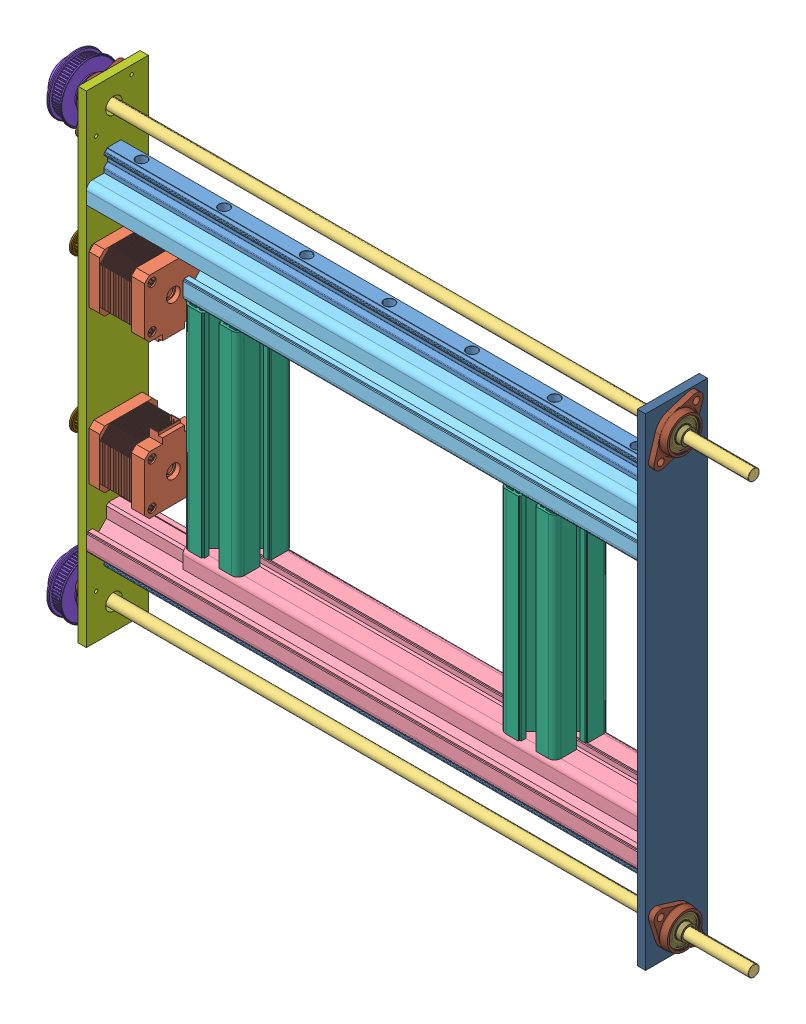
SolidWorks assembly Mesa, configuration Predeterminado. Lengths in mm.
Overall size (500 363.97 51.97).
38 component instances, 15 part files, 62 mates.
Components (placement in the parent):
- Mesa-1: Mesa [Predeterminado] at origin size (412 330 4) (hidden)
- Copia de HGR15R Rail^Mesa-1: Copia de HGR15R Rail^Mesa [HGR15R400CE20] at (0 282 -20) x (0 0 1) z (-1 0 0) size (15 15 400) (virtual)
- Copia de HGR15R Rail^Mesa-2: Copia de HGR15R Rail^Mesa [HGR15R400CE20] at (0 48 -20) x (0 0 -1) z (-1 0 0) size (15 15 400) (virtual)
- Nema_17HS4401-S^Mesa-1: Nema_17HS4401-S^Mesa [Varsayılan] at (40.2 220.5 -23) x (0 0 -1) z (-1 0 0) size (42 48 63.23) (virtual)
- LeadScrew 8mm x 2mmPitch^Mesa-1: LeadScrew 8mm x 2mmPitch^Mesa [Default] at (464.65 9 -20) x (0 1 0) z (1 0 0) size (8 8 500) (virtual)
- LeadScrew 8mm x 2mmPitch^Mesa-2: LeadScrew 8mm x 2mmPitch^Mesa [Default] at (464.65 321 -20) x (0 -1 0) z (1 0 0) size (8 8 500) (virtual)
- yn_4040^Mesa-1: yn_4040^Mesa [Default] at (400 68 -20) x (0 1 0) z (-1 0 0) size (40 40 400) (virtual)
- yp_4040^Mesa-3: yp_4040^Mesa [Default] at (400 262 -20) x (0 1 0) z (-1 0 0) size (40 40 400) (virtual)
- xp_4040^Mesa-2: xp_4040^Mesa [Default] at (90 242 -20) x (-1 0 0) z (0 -1 0) size (40 40 154) (virtual)
- soporte_motores^Mesa-1: soporte_motores^Mesa [Predeterminado] at (-6 340 0) x (0 1 0) z (1 0 0) size (350 45 6) (virtual)
- farola^Mesa-1: farola^Mesa [Predeterminado] at (450.1962 5.1009 28.2108) x (0.008727 0.999962 0) z (0 0 1) size (325 500 6) (hidden, virtual)
- GT2_60T_8_6^Mesa-2: GT2_60T_8_6^Mesa [Default] at (-27.85 321 -20) x (0 0 1) z (1 0 0) size (42 42 18) (virtual)
- GT2_20T^Mesa-1: GT2_20T^Mesa [Конфигурация1] at (-11.4 220.5 -23) x (-1 0 0) z (0 0 1) size (16 16 16) (virtual)
- GT2_60T_8_6^Mesa-3: GT2_60T_8_6^Mesa [Default] at (-27.85 9 -20) x (0 0 -1) z (1 0 0) size (42 42 18) (virtual)
- Nema_17HS4401-S^Mesa-2: Nema_17HS4401-S^Mesa [Varsayılan] at (40.2 109.5 -23) x (0 0 1) z (-1 0 0) size (42 48 63.23) (virtual)
- GT2_20T^Mesa-2: GT2_20T^Mesa [Конфигурация1] at (-11.4 109.5 -23) x (-1 0 0) z (0 1 0) size (16 16 16) (virtual)
- soporte_frontal^Mesa-1: soporte_frontal^Mesa [Predeterminado] at (400 340 0) x (0 1 0) z (1 0 0) size (350 45 6) (virtual)
- KFL08^Mesa-3: KFL08^Mesa [Varsayılan] at (-6 9 -20) x (0 0.707107 0.707107) z (0 -0.707107 0.707107) size (46.5 11.35 27) (virtual)
  - FLANGE-1: FLANGE [Default] at origin size (46.5 8.5 27)
  - BEARING-1: BEARING [Default] at (0 4 0) x (1 0 0) z (0 -1 0) size (22 22 10.85)
  - socket set screw cone point_am-1: socket set screw cone point_am [B18.3.6M - M2.5 x 0.45 x 2 Hex Socket Cone Pt. SS --S] at (0 9.425 5.45) x (0 0 -1) z (1 0 0) size (2 2.5 2.5)
  - socket set screw cone point_am-2: socket set screw cone point_am [B18.3.6M - M2.5 x 0.45 x 2 Hex Socket Cone Pt. SS --S] at (5.45 9.425 0) x (-1 0 0) z (0 0 -1) size (2 2.5 2.5)
- KFL08^Mesa-2: KFL08^Mesa [Varsayılan] at (-6 321 -20) x (0 -0.707107 0.707107) z (0 -0.707107 -0.707107) size (46.5 11.35 27) (virtual)
  - FLANGE-1: FLANGE [Default] at origin size (46.5 8.5 27)
  - BEARING-1: BEARING [Default] at (0 4 0) x (1 0 0) z (0 -1 0) size (22 22 10.85)
  - socket set screw cone point_am-1: socket set screw cone point_am [B18.3.6M - M2.5 x 0.45 x 2 Hex Socket Cone Pt. SS --S] at (0 9.425 5.45) x (0 0 -1) z (1 0 0) size (2 2.5 2.5)
  - socket set screw cone point_am-2: socket set screw cone point_am [B18.3.6M - M2.5 x 0.45 x 2 Hex Socket Cone Pt. SS --S] at (5.45 9.425 0) x (-1 0 0) z (0 0 -1) size (2 2.5 2.5)
- KFL08^Mesa-4: KFL08^Mesa [Varsayılan] at (406 9 -20) x (0 -0.707107 -0.707107) z (0 -0.707107 0.707107) size (46.5 11.35 27) (virtual)
  - FLANGE-1: FLANGE [Default] at origin size (46.5 8.5 27)
  - BEARING-1: BEARING [Default] at (0 4 0) x (1 0 0) z (0 -1 0) size (22 22 10.85)
  - socket set screw cone point_am-1: socket set screw cone point_am [B18.3.6M - M2.5 x 0.45 x 2 Hex Socket Cone Pt. SS --S] at (0 9.425 5.45) x (0 0 -1) z (1 0 0) size (2 2.5 2.5)
  - socket set screw cone point_am-2: socket set screw cone point_am [B18.3.6M - M2.5 x 0.45 x 2 Hex Socket Cone Pt. SS --S] at (5.45 9.425 0) x (-1 0 0) z (0 0 -1) size (2 2.5 2.5)
- KFL08^Mesa-5: KFL08^Mesa [Varsayılan] at (406 321 -20) x (0 0.707107 -0.707107) z (0 -0.707107 -0.707107) size (46.5 11.35 27) (virtual)
  - FLANGE-1: FLANGE [Default] at origin size (46.5 8.5 27)
  - BEARING-1: BEARING [Default] at (0 4 0) x (1 0 0) z (0 -1 0) size (22 22 10.85)
  - socket set screw cone point_am-1: socket set screw cone point_am [B18.3.6M - M2.5 x 0.45 x 2 Hex Socket Cone Pt. SS --S] at (0 9.425 5.45) x (0 0 -1) z (1 0 0) size (2 2.5 2.5)
  - socket set screw cone point_am-2: socket set screw cone point_am [B18.3.6M - M2.5 x 0.45 x 2 Hex Socket Cone Pt. SS --S] at (5.45 9.425 0) x (-1 0 0) z (0 0 -1) size (2 2.5 2.5)
- xp_4040^Mesa-3: xp_4040^Mesa [Default] at (320 242 -20) x (-1 0 0) z (0 -1 0) size (40 40 154) (virtual)
Mates (geometry in assembly coordinates):
- Coincidente34: coincident anti-aligned: plane of Mesa-1 through (0 0 0) normal (0 0 -1); plane of yn_4040^Mesa-1 through (0 52.5 0) normal (0 0 1)
- Coincidente35: coincident aligned: plane of Mesa-1 through (0 0 4) normal (-1 0 0); plane of yn_4040^Mesa-1 through (0 83.5 -35.5) normal (-1 0 0)
- Coincidente36: coincident anti-aligned: plane of Mesa-1 through (0 0 0) normal (0 0 -1); plane of yp_4040^Mesa-3 through (0 246.5 0) normal (0 0 1)
- Coincidente37: coincident aligned: plane of Mesa-1 through (0 0 4) normal (-1 0 0); plane of yp_4040^Mesa-3 through (0 277.5 -35.5) normal (-1 0 0)
- Coincidente38: coincident anti-aligned: plane of Copia de HGR15R Rail^Mesa-2 through (400 48 -13) normal (0 1 0); plane of yn_4040^Mesa-1 through (0 48 -23.9656) normal (0 -1 0)
- Coincidente39: coincident aligned: plane of Copia de HGR15R Rail^Mesa-2 through (0 44.9142 -26.5) normal (-1 0 0); plane of yn_4040^Mesa-1 through (0 83.5 -35.5) normal (-1 0 0)
- Coincidente40: coincident anti-aligned: plane of Copia de HGR15R Rail^Mesa-1 through (400 282 -27) normal (0 -1 0); plane of yp_4040^Mesa-3 through (0 282 -23.9656) normal (0 1 0)
- Coincidente41: coincident aligned: plane of Copia de HGR15R Rail^Mesa-1 through (0 285.0858 -13.5) normal (-1 0 0); plane of yp_4040^Mesa-3 through (0 277.5 -35.5) normal (-1 0 0)
- Distancia9: distance = 12.5 mm aligned: plane of Copia de HGR15R Rail^Mesa-1 through (400 282.5 -27.5) normal (0 0 -1); plane of yp_4040^Mesa-3 through (0 277.5 -40) normal (0 0 -1)
- Distancia10: distance = 12.5 mm aligned: plane of Copia de HGR15R Rail^Mesa-2 through (400 47.5 -27.5) normal (0 0 -1); plane of yn_4040^Mesa-1 through (0 52.5 -40) normal (0 0 -1)
- Distancia13: distance = 48 mm aligned: plane of yn_4040^Mesa-1 through (0 48 -16.0344) normal (0 -1 0); plane of Mesa-1 through (0 0 4) normal (0 -1 0)
- Distancia15: distance = 154 mm anti-aligned: plane of yn_4040^Mesa-1 through (0 88 -16.0344) normal (0 1 0); plane of yp_4040^Mesa-3 through (0 242 -16.0344) normal (0 -1 0)
- Coincidente49: coincident anti-aligned: plane of yp_4040^Mesa-3 through (0 277.5 -35.5) normal (-1 0 0); plane of soporte_motores^Mesa-1 through (0 340 0) normal (1 0 0)
- Coincidente50: coincident aligned: plane of yp_4040^Mesa-3 through (0 277.5 0) normal (0 0 1); plane of soporte_motores^Mesa-1 through (0 -10 0) normal (0 0 1)
- Distancia18: distance = 58 mm aligned: plane of yp_4040^Mesa-3 through (0 282 -16.0344) normal (0 1 0); plane of soporte_motores^Mesa-1 through (0 340 -45) normal (0 1 0)
- Coincidente52: coincident anti-aligned: plane of soporte_motores^Mesa-1 through (-6 340 0) normal (-1 0 0); plane of KFL08^Mesa-2/FLANGE-1 through (-6 308.0953 -7.0953) normal (1 0 0)
- Concéntrica1: concentric aligned: cylinder of soporte_motores^Mesa-1 through (-6 321 -20) axis (1 0 0) radius 6; cylinder of KFL08^Mesa-2/BEARING-1 through (-6.5 321 -20) axis (1 0 0) radius 4
- Concéntrica2: concentric anti-aligned: cylinder of soporte_motores^Mesa-1 through (-6 333.9047 -32.9047) axis (1 0 0) radius 1.25; cylinder of KFL08^Mesa-2/FLANGE-1 through (-10 333.9047 -32.9047) axis (-1 0 0) radius 2.5
- Coincidente53: coincident anti-aligned: plane of soporte_motores^Mesa-1 through (-6 340 0) normal (-1 0 0); plane of KFL08^Mesa-3/FLANGE-1 through (-6 21.9047 -7.0953) normal (1 0 0)
- Concéntrica3: concentric aligned: cylinder of soporte_motores^Mesa-1 through (-6 9 -20) axis (1 0 0) radius 6; cylinder of KFL08^Mesa-3/BEARING-1 through (-6.5 9 -20) axis (1 0 0) radius 4
- Concéntrica4: concentric anti-aligned: cylinder of soporte_motores^Mesa-1 through (-6 21.9047 -7.0953) axis (1 0 0) radius 1.25; cylinder of KFL08^Mesa-3/FLANGE-1 through (-10 21.9047 -7.0953) axis (-1 0 0) radius 2.5
- Concéntrica5: concentric aligned: cylinder of LeadScrew 8mm x 2mmPitch^Mesa-1 through (-35.35 9 -20) axis (1 0 0) radius 4; cylinder of KFL08^Mesa-3/BEARING-1 through (-6.5 9 -20) axis (1 0 0) radius 4
- Concéntrica6: concentric aligned: cylinder of LeadScrew 8mm x 2mmPitch^Mesa-2 through (-35.35 321 -20) axis (1 0 0) radius 4; cylinder of KFL08^Mesa-2/BEARING-1 through (-6.5 321 -20) axis (1 0 0) radius 4
- Concéntrica7: concentric aligned: circle of LeadScrew 8mm x 2mmPitch^Mesa-2; circle of GT2_60T_8_6^Mesa-2
- Coincidente54: coincident anti-aligned: plane of KFL08^Mesa-2/BEARING-1 through (-17.35 317.9594 -23.0406) normal (-1 0 0); plane of GT2_60T_8_6^Mesa-2 through (-17.35 321 -20) normal (1 0 0)
- Coincidente55: coincident aligned: plane of LeadScrew 8mm x 2mmPitch^Mesa-2 through (-35.35 321 -20) normal (-1 0 0); plane of GT2_60T_8_6^Mesa-2 through (-35.35 321 -20) normal (-1 0 0)
- Coincidente56: coincident anti-aligned: plane of Nema_17HS4401-S^Mesa-1 through (0 220.5 -23) normal (-1 0 0); plane of soporte_motores^Mesa-1 through (0 340 0) normal (1 0 0)
- Distancia19: distance = 2 mm aligned: plane of Nema_17HS4401-S^Mesa-1 through (30.7 238 -2) normal (0 0 1); plane of soporte_motores^Mesa-1 through (0 -10 0) normal (0 0 1)
- Distancia20: distance = 15 mm anti-aligned: plane of Nema_17HS4401-S^Mesa-1 through (30.7 241.5 -5.5) normal (0 1 0); plane of yp_4040^Mesa-3 through (0 256.5 -20) normal (0 -1 0)
- Concéntrica8: concentric anti-aligned: cylinder of Nema_17HS4401-S^Mesa-1 through (-23 220.5 -23) axis (1 0 0) radius 2.5; cylinder of GT2_20T^Mesa-1 through (-11.4 220.5 -23) axis (-1 0 0) radius 2.5
- Coincidente59: coincident aligned: plane of GT2_60T_8_6^Mesa-2 through (-18.85 321 -20) normal (-1 0 0); plane of GT2_20T^Mesa-1 through (-18.85 220.5 -23) normal (-1 0 0)
- Concéntrica9: concentric anti-aligned: cylinder of LeadScrew 8mm x 2mmPitch^Mesa-1 through (-35.35 9 -20) axis (1 0 0) radius 4; cylinder of GT2_60T_8_6^Mesa-3 through (2.15 9 -20) axis (-1 0 0) radius 4
- Coincidente60: coincident anti-aligned: plane of KFL08^Mesa-3/BEARING-1 through (-17.35 5.9594 -16.9594) normal (-1 0 0); plane of GT2_60T_8_6^Mesa-3 through (-17.35 9 -20) normal (1 0 0)
- Coincidente61: coincident aligned: plane of LeadScrew 8mm x 2mmPitch^Mesa-1 through (-35.35 9 -20) normal (-1 0 0); plane of GT2_60T_8_6^Mesa-3 through (-35.35 9 -20) normal (-1 0 0)
- Coincidente62: coincident anti-aligned: plane of soporte_motores^Mesa-1 through (0 340 0) normal (1 0 0); plane of Nema_17HS4401-S^Mesa-2 through (0 109.5 -23) normal (-1 0 0)
- Distancia21: distance = 15 mm anti-aligned: plane of Nema_17HS4401-S^Mesa-2 through (30.7 88.5 -40.5) normal (0 -1 0); plane of yn_4040^Mesa-1 through (0 73.5 -20) normal (0 1 0)
- Distancia22: distance = 2 mm aligned: plane of Nema_17HS4401-S^Mesa-2 through (30.7 92 -2) normal (0 0 1); plane of soporte_motores^Mesa-1 through (0 -10 0) normal (0 0 1)
- Concéntrica10: concentric anti-aligned: cylinder of Nema_17HS4401-S^Mesa-2 through (-23 109.5 -23) axis (1 0 0) radius 2.5; cylinder of GT2_20T^Mesa-2 through (-11.4 109.5 -23) axis (-1 0 0) radius 2.5
- Coincidente65: coincident aligned: plane of GT2_60T_8_6^Mesa-3 through (-18.85 9 -20) normal (-1 0 0); plane of GT2_20T^Mesa-2 through (-18.85 109.5 -23) normal (-1 0 0)
- Coincidente66: coincident anti-aligned: plane of yn_4040^Mesa-1 through (400 83.5 -35.5) normal (1 0 0); plane of soporte_frontal^Mesa-1 through (400 340 0) normal (-1 0 0)
- Coincidente67: coincident aligned: plane of yn_4040^Mesa-1 through (0 52.5 0) normal (0 0 1); plane of soporte_frontal^Mesa-1 through (406 -10 0) normal (0 0 1)
- Concéntrica11: concentric aligned: cylinder of LeadScrew 8mm x 2mmPitch^Mesa-1 through (-35.35 9 -20) axis (1 0 0) radius 4; cylinder of soporte_frontal^Mesa-1 through (400 9 -20) axis (1 0 0) radius 6
- Coincidente68: coincident anti-aligned: plane of soporte_frontal^Mesa-1 through (406 340 0) normal (1 0 0); plane of KFL08^Mesa-5/FLANGE-1 through (406 333.9047 -32.9047) normal (-1 0 0)
- Coincidente69: coincident anti-aligned: plane of soporte_frontal^Mesa-1 through (406 340 0) normal (1 0 0); plane of KFL08^Mesa-4/FLANGE-1 through (406 -3.9047 -32.9047) normal (-1 0 0)
- Concéntrica12: concentric aligned: cylinder of soporte_frontal^Mesa-1 through (400 21.9047 -7.0953) axis (1 0 0) radius 1.25; cylinder of KFL08^Mesa-4/FLANGE-1 through (410 21.9047 -7.0953) axis (1 0 0) radius 2.5
- Concéntrica13: concentric anti-aligned: cylinder of LeadScrew 8mm x 2mmPitch^Mesa-1 through (-35.35 9 -20) axis (1 0 0) radius 4; cylinder of KFL08^Mesa-4/BEARING-1 through (406.5 9 -20) axis (-1 0 0) radius 4
- Concéntrica14: concentric anti-aligned: cylinder of LeadScrew 8mm x 2mmPitch^Mesa-2 through (-35.35 321 -20) axis (1 0 0) radius 4; cylinder of KFL08^Mesa-5/BEARING-1 through (406.5 321 -20) axis (-1 0 0) radius 4
- Concéntrica15: concentric aligned: cylinder of soporte_frontal^Mesa-1 through (400 308.0953 -7.0953) axis (1 0 0) radius 1.25; cylinder of KFL08^Mesa-5/FLANGE-1 through (410 308.0953 -7.0953) axis (1 0 0) radius 2.5
- Paralelo1: parallel aligned: plane of LeadScrew 8mm x 2mmPitch^Mesa-1 through (-25.35 6 -13.5951) normal (0 -1 0); plane of GT2_60T_8_6^Mesa-3 through (-31.6 -4 -20) normal (0 -1 0)
- Paralelo2: parallel aligned: plane of soporte_motores^Mesa-1 through (0 -10 -45) normal (0 -1 0); plane of GT2_60T_8_6^Mesa-3 through (-31.6 -4 -20) normal (0 -1 0)
- Paralelo3: parallel aligned: plane of LeadScrew 8mm x 2mmPitch^Mesa-2 through (-25.35 324 -26.4049) normal (0 1 0); plane of GT2_60T_8_6^Mesa-2 through (-31.6 334 -20) normal (0 1 0)
- Paralelo4: parallel aligned: plane of soporte_motores^Mesa-1 through (0 340 -45) normal (0 1 0); plane of GT2_60T_8_6^Mesa-2 through (-31.6 334 -20) normal (0 1 0)
- Paralelo5: parallel aligned: plane of Nema_17HS4401-S^Mesa-1 through (-6 218.6296 -21.3412) normal (0 -1 0); plane of GT2_20T^Mesa-1 through (-15.4 213 -23) normal (0 -1 0)
- Paralelo6: parallel aligned: plane of soporte_motores^Mesa-1 through (0 -10 0) normal (0 0 1); plane of GT2_20T^Mesa-1 through (-15.4 220.5 -15.5) normal (0 0 1)
- Paralelo7: parallel aligned: plane of Nema_17HS4401-S^Mesa-2 through (-6 111.3704 -24.6588) normal (0 1 0); plane of GT2_20T^Mesa-2 through (-15.4 117 -23) normal (0 1 0)
- Paralelo8: parallel aligned: plane of soporte_motores^Mesa-1 through (0 -10 0) normal (0 0 1); plane of GT2_20T^Mesa-2 through (-15.4 109.5 -15.5) normal (0 0 1)
- Coincidente76: coincident anti-aligned: plane of yp_4040^Mesa-3 through (0 242 -16.0344) normal (0 -1 0); plane of xp_4040^Mesa-2 through (74.5 242 -35.5) normal (0 1 0)
- Coincidente77: coincident aligned: plane of yp_4040^Mesa-3 through (0 246.5 0) normal (0 0 1); plane of xp_4040^Mesa-2 through (105.5 88 0) normal (0 0 1)
- Distancia23: distance = 70 mm anti-aligned: plane of soporte_motores^Mesa-1 through (0 340 0) normal (1 0 0); plane of xp_4040^Mesa-2 through (70 88 -16.0344) normal (-1 0 0)
- Coincidente79: coincident aligned: plane of yp_4040^Mesa-3 through (0 246.5 0) normal (0 0 1); plane of xp_4040^Mesa-3 through (335.5 88 0) normal (0 0 1)
- Coincidente80: coincident anti-aligned: plane of yp_4040^Mesa-3 through (0 242 -16.0344) normal (0 -1 0); plane of xp_4040^Mesa-3 through (304.5 242 -35.5) normal (0 1 0)
- Distancia24: distance = 60 mm anti-aligned: plane of xp_4040^Mesa-3 through (340 88 -16.0344) normal (1 0 0); plane of soporte_frontal^Mesa-1 through (400 340 0) normal (-1 0 0)
